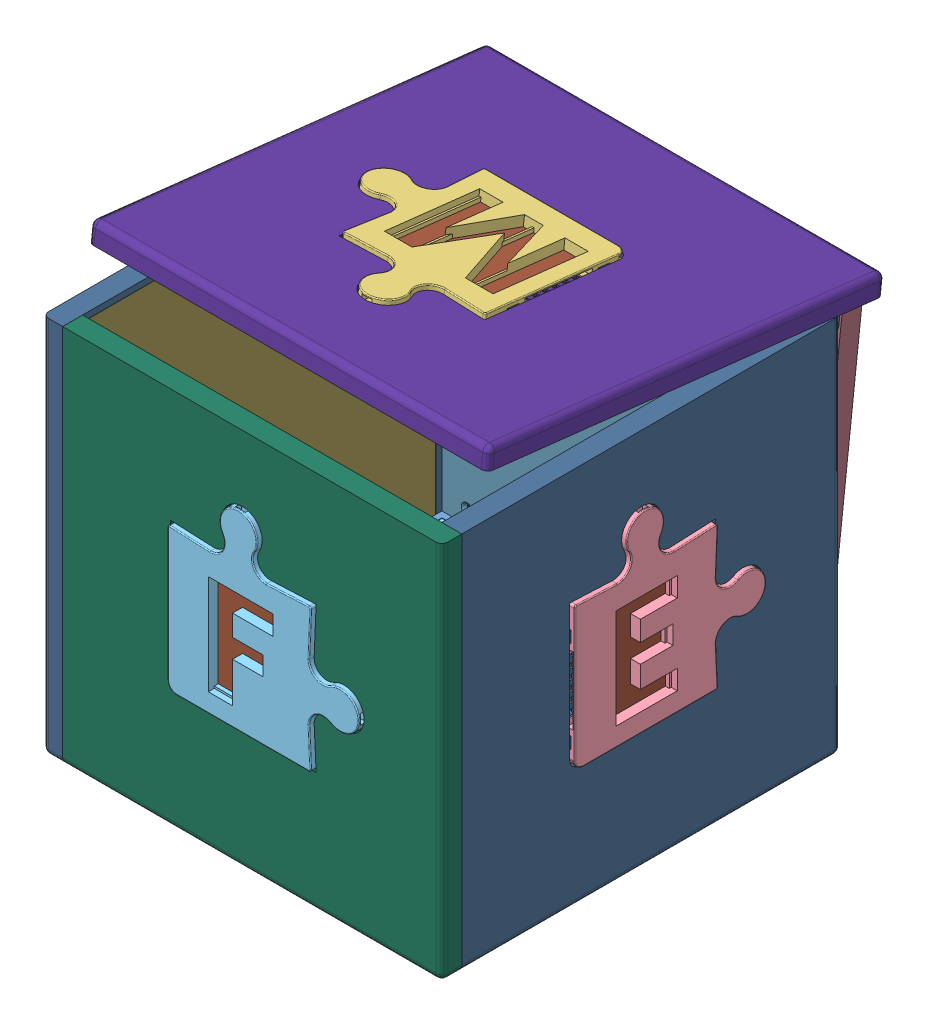
SolidWorks assembly new_full_ass, configuration Default. Lengths in mm.
Overall size (204.06 222.93 226.17).
48 component instances, 23 part files, 47 mates.
Components (placement in the parent):
- base_ass-1: base_ass [Default] at (110.6149 77.5373 125.031) size (180 19.96 180)
  - base-1: base [Default] at (-36.6134 -12.1869 24.2031) size (180 15 180)
  - speaker-2: speaker [Default] at (18.5866 0.8131 47.2031) x (0 0 -1) z (-1 0 0) size (40 8 20)
  - type-c_BMS_module-2: type-c_BMS_module [Default] at (27.2366 -9.1869 112.2031) x (0 0 -1) z (0 1 0) size (29.08 17.3 4.86)
  - battery-2: battery [Default] at (-36.6134 -10.1869 -24.7969) size (132 12 42)
  - tutup_base-1: tutup_base [Default] at (-36.6134 0.8131 24.2031) size (173.5 12 173.5)
  - switch-1: switch [Default] at (-5.9134 -5.1869 89.9531) size (10 14.96 15)
  - smart_puzzle-1: smart_puzzle [Default] at (19.033 -5.5869 172.5712) x (0 0 -1) z (0 1 0) size (76.84 76.96 8.3)
- hinge-1: hinge [Default] at (104.8865 81.1552 217.17) x (0 -1 0) z (-1 0 0) size (11.5 5 40) (flexible)
  - hinge_A-1: hinge_A [Default] at (15.8048 19.5641 50.885) size (11.5 5 40)
  - hinge_B-1: hinge_B [Default] at (6.8048 24.5641 50.885) x (-1 0 0) z (0 0 1) size (11.5 5 40)
- hinge-2: hinge [Default] at (6.0656 81.1552 180.1191) x (0 -1 0) z (0 0 -1) size (11.5 5 40) (flexible)
  - hinge_A-1: hinge_A [Default] at (15.8048 19.5641 50.885) size (11.5 5 40)
  - hinge_B-1: hinge_B [Default] at (6.8048 24.5641 50.885) x (-1 0 0) z (0 0 1) size (11.5 5 40)
- hinge-3: hinge [Default] at (43.1164 81.1552 81.2982) x (0 -1 0) z (1 0 0) size (11.99 6.27 40) (flexible)
  - hinge_A-1: hinge_A [Default] at (15.8048 19.5641 50.885) size (11.5 5 40)
  - hinge_B-1: hinge_B [Default] at (7.1444 25.5637 50.885) x (-0.993614 0.112837 0) z (0 0 1) size (11.5 5 40)
- hinge-4: hinge [Default] at (141.9374 81.1552 118.3491) x (0 -1 0) z (0 0 1) size (11.5 5 40) (flexible)
  - hinge_A-1: hinge_A [Default] at (15.8048 19.5641 50.885) size (11.5 5 40)
  - hinge_B-1: hinge_B [Default] at (6.8048 24.5641 50.885) x (-1 0 0) z (0 0 1) size (11.5 5 40)
- side_ass-2: side_ass [Default] at (-27.75 544.2015 -410.629) x (0 0 -1) z (0 -1 0) size (190 10 190)
  - side-1: side [Default] at (-559.8631 11.7515 383.8511) x (0 -1 0) z (-1 0 0) size (10 190 190)
  - RGB_backlight-1: RGB_backlight [Default] at (-559.8631 6.7515 383.8511) x (-1 0 0) z (0 0 -1) size (71 3 80)
  - tutup_side-1: tutup_side [Default] at (-564.8631 9.7515 389.9511) x (-1 0 0) z (0 0 -1) size (185.8 2 183.8)
- side_ass-3: side_ass [Default] at (175.7529 544.2015 709.0972) x (0 0 1) z (0 -1 0) size (190 10 190)
  - side-1: side [Default] at (-559.8631 11.7515 383.8511) x (0 -1 0) z (-1 0 0) size (10 190 190)
  - RGB_backlight-1: RGB_backlight [Default] at (-559.8631 6.7515 383.8511) x (-1 0 0) z (0 0 -1) size (71 3 80)
  - tutup_side-1: tutup_side [Default] at (-564.8631 9.7515 389.9511) x (-1 0 0) z (0 0 -1) size (185.8 2 183.8)
- side_top_hinge_ass-1: side_top_hinge_ass [Default] at (71.9264 168.2711 22.0939) x (0 -0.112837 -0.993614) z (-1 0 0) size (10 190 190)
  - side_top_hinge-1: side_top_hinge [Default] at (-25.2898 11.4541 -2.0751) size (10 190 190)
  - tutup_side_top_hinge-1: tutup_side_top_hinge [Default] at (-23.2898 11.4541 2.9249) x (0 0 1) z (0 -1 0) size (185.5 2 183.5)
  - RGB_backlight-1: RGB_backlight [Default] at (-23.2898 11.4541 -2.0751) x (0 0 -1) z (0 -1 0) size (71 3 80)
- side_top_magnet_ass-1: side_top_magnet_ass [Default] at (71.9462 160.3504 257.6043) x (0 0 1) z (1 0 0) size (10 190 190)
  - side_top_magnet-1: side_top_magnet [Default] at (-18.3702 0 2.0553) size (10 190 190)
  - RGB_backlight-1: RGB_backlight [Default] at (-13.3702 0 2.0553) x (0 0 1) z (0 -1 0) size (71 3 80)
  - tutup_side_top_magnet-1: tutup_side_top_magnet [Default] at (-16.3702 0 7.0553) x (0 0 1) z (0 -1 0) size (185.5 2 185.5)
- hinge-5: hinge [Default] at (43.1164 232.8688 46.0525) x (0 -0.112837 -0.993614) z (1 0 0) size (11.5 5 40) (flexible)
  - hinge_A-1: hinge_A [Default] at (15.8048 19.5641 50.885) size (11.5 5 40)
  - hinge_B-1: hinge_B [Default] at (6.8048 24.5641 50.885) x (-1 0 0) z (0 0 1) size (11.5 5 40)
- top_ass-1: top_ass [Default] at (54.7211 254.2163 143.7349) x (0 0.993614 -0.112837) z (-1 0 0) size (10 200 200)
  - top-1: top [Default] at (11.8751 15.2721 -19.2804) size (10 200 200)
  - tutup_top-1: tutup_top [Default] at (13.8751 15.2721 -19.2804) x (0 0 1) z (0 -1 0) size (195.5 2 193.5)
  - RGB_backlight-1: RGB_backlight [Default] at (16.8751 15.2721 -19.2804) x (0 0 1) z (0 -1 0) size (71 3 80)
- A-1: A [Default] at (-22.9985 161.3504 149.2341) x (0 0 1) z (0 -1 0) size (95.8 5.06 95.8)
- H-1: H [Default] at (74.0015 159.9475 41.4465) x (-1 0 0) z (0 -0.993614 0.112837) size (95.8 5.06 95.8)
- M-1: M [Default] at (74.0015 271.3604 127.4241) x (-1 0 0) z (0 -0.112837 -0.993614) size (95.8 5.06 95.8)
- E-1: E [Default] at (171.0015 161.3504 149.2341) x (0 0 -1) z (0 -1 0) size (95.8 5.06 95.8)
- N-1: N [Default] at (74.0015 161.3504 246.2341) x (1 0 0) z (0 -1 0) size (95.8 5.06 95.8)
Mates (geometry in assembly coordinates):
- Coincident1: coincident anti-aligned: line of base_ass-1/base-1 through (94.4015 65.3504 239.2341) axis (1 0 0); line of hinge-1 through (91.3609 65.3504 239.2341) axis (-1 0 0)
- Parallel1: parallel anti-aligned: plane of base_ass-1/base-1 through (74.0015 65.3504 236.6341) normal (0 0 1); plane of hinge-1/hinge_A-1 through (54.0015 65.3504 236.7341) normal (0 0 -1)
- Width1: width anti-aligned: plane of base_ass-1/base-1 through (53.6015 65.3504 236.6341) normal (1 0 0); plane of hinge-1/hinge_A-1 through (94.4015 65.3504 236.6341) normal (-1 0 0); plane of base_ass-1/base-1 through (54.0015 74.3504 239.2341) normal (-1 0 0); plane of hinge-1/hinge_A-1 through (94.0015 74.3504 239.2341) normal (1 0 0)
- Coincident3: coincident anti-aligned: line of base_ass-1/base-1 through (-15.9985 65.3504 59.2341) axis (0 0 1); line of hinge-2 through (-15.9985 65.3504 166.5936) axis (0 0 -1)
- Parallel2: parallel anti-aligned: plane of base_ass-1/base-1 through (-13.3985 65.3504 149.2341) normal (-1 0 0); plane of hinge-2/hinge_A-1 through (-13.4985 65.3504 129.2341) normal (1 0 0)
- Width2: width anti-aligned: plane of base_ass-1/base-1 through (-13.3985 65.3504 128.8341) normal (0 0 1); plane of hinge-2/hinge_A-1 through (-13.3985 65.3504 169.6341) normal (0 0 -1); plane of base_ass-1/base-1 through (-15.9985 74.3504 129.2341) normal (0 0 -1); plane of hinge-2/hinge_A-1 through (-15.9985 74.3504 169.2341) normal (0 0 1)
- Coincident5: coincident aligned: line of base_ass-1/base-1 through (94.4015 65.3504 59.2341) axis (1 0 0); line of hinge-3 through (56.642 65.3504 59.2341) axis (1 0 0)
- Parallel3: parallel anti-aligned: plane of base_ass-1/base-1 through (74.0015 65.3504 61.8341) normal (0 0 -1); plane of hinge-3/hinge_A-1 through (94.0015 65.3504 61.7341) normal (0 0 1)
- Width3: width anti-aligned: plane of base_ass-1/base-1 through (94.4015 65.3504 61.8341) normal (-1 0 0); plane of hinge-3/hinge_A-1 through (53.6015 65.3504 61.8341) normal (1 0 0); plane of base_ass-1/base-1 through (94.0015 74.3504 59.2341) normal (1 0 0); plane of hinge-3/hinge_A-1 through (54.0015 74.3504 59.2341) normal (-1 0 0)
- Coincident11: coincident aligned: line of base_ass-1/base-1 through (164.0015 65.3504 169.6341) axis (0 0 1); line of hinge-4 through (164.0015 65.3504 131.8746) axis (0 0 1)
- Width4: width anti-aligned: plane of base_ass-1/base-1 through (161.4015 65.3504 128.8341) normal (0 0 1); plane of hinge-4/hinge_A-1 through (161.4015 65.3504 169.6341) normal (0 0 -1); plane of base_ass-1/base-1 through (164.0015 74.3504 129.2341) normal (0 0 -1); plane of hinge-4/hinge_A-1 through (164.0015 74.3504 169.2341) normal (0 0 1)
- Parallel5: parallel anti-aligned: plane of base_ass-1/base-1 through (161.4015 65.3504 149.2341) normal (1 0 0); plane of hinge-4/hinge_A-1 through (161.5015 65.3504 169.2341) normal (-1 0 0)
- Width5: width anti-aligned: plane of side_ass-2/side-1 through (-18.5985 65.3504 128.8341) normal (0 0 1); plane of hinge-2/hinge_B-1 through (-18.5985 65.3504 169.6341) normal (0 0 -1); plane of side_ass-2/side-1 through (-15.9985 74.3504 129.2341) normal (0 0 -1); plane of hinge-2/hinge_B-1 through (-15.9985 74.3504 169.2341) normal (0 0 1)
- Parallel6: parallel anti-aligned: plane of hinge-2/hinge_B-1 through (-18.4985 74.3504 129.2341) normal (-1 0 0); plane of side_ass-2/side-1 through (-18.5985 160.3504 149.2341) normal (1 0 0)
- Coincident12: coincident aligned: line of base_ass-1/base-1 through (-15.9985 65.3504 169.6341) axis (0 0 1); line of side_ass-2/side-1 through (-15.9985 65.3504 169.6341) axis (0 0 1)
- Width6: width anti-aligned: plane of side_ass-3/side-1 through (166.6015 65.3504 128.8341) normal (0 0 1); plane of hinge-4/hinge_B-1 through (166.6015 65.3504 169.6341) normal (0 0 -1); plane of side_ass-3/side-1 through (164.0015 74.3504 129.2341) normal (0 0 -1); plane of hinge-4/hinge_B-1 through (164.0015 74.3504 169.2341) normal (0 0 1)
- Parallel7: parallel anti-aligned: plane of hinge-4/hinge_B-1 through (166.5015 74.3504 169.2341) normal (1 0 0); plane of side_ass-3/side-1 through (166.6015 160.3504 149.2341) normal (-1 0 0)
- Coincident14: coincident anti-aligned: line of base_ass-1/base-1 through (164.0015 65.3504 169.6341) axis (0 0 1); line of side_ass-3/side-1 through (164.0015 65.3504 239.2341) axis (0 0 -1)
- Width7: width anti-aligned: plane of side_top_hinge_ass-1/side_top_hinge-1 through (94.4015 65.0571 56.6507) normal (-1 0 0); plane of hinge-3/hinge_B-1 through (53.6015 65.0571 56.6507) normal (1 0 0); plane of side_top_hinge_ass-1/side_top_hinge-1 through (94.0015 74.293 58.2186) normal (1 0 0); plane of hinge-3/hinge_B-1 through (54.0015 74.293 58.2186) normal (-1 0 0)
- Parallel8: parallel anti-aligned: plane of hinge-3/hinge_B-1 through (94.0015 74.0109 55.7345) normal (0 -0.112837 -0.993614); plane of side_top_hinge_ass-1/side_top_hinge-1 through (74.0015 159.4503 45.9312) normal (0 0.112837 0.993614)
- Coincident16: coincident anti-aligned: line of base_ass-1/base-1 through (-15.9985 65.3504 59.2341) axis (1 0 0); line of side_top_hinge_ass-1/side_top_hinge-1 through (53.6015 65.3504 59.2341) axis (-1 0 0)
- Width8: width anti-aligned: plane of side_top_magnet_ass-1/side_top_magnet-1 through (94.4015 65.3504 241.8341) normal (-1 0 0); plane of hinge-1/hinge_B-1 through (53.6015 65.3504 241.8341) normal (1 0 0); plane of side_top_magnet_ass-1/side_top_magnet-1 through (94.0015 74.3504 239.2341) normal (1 0 0); plane of hinge-1/hinge_B-1 through (54.0015 74.3504 239.2341) normal (-1 0 0)
- Parallel9: parallel anti-aligned: plane of hinge-1/hinge_B-1 through (54.0015 74.3504 241.7341) normal (0 0 1); plane of side_top_magnet_ass-1/side_top_magnet-1 through (74.0015 160.3504 241.8341) normal (0 0 -1)
- Coincident17: coincident aligned: line of base_ass-1/base-1 through (-15.9985 65.3504 239.2341) axis (1 0 0); line of side_top_magnet_ass-1/side_top_magnet-1 through (-15.9985 65.3504 239.2341) axis (1 0 0)
- Width9: width anti-aligned: plane of side_top_hinge_ass-1/side_top_hinge-1 through (94.4015 251.4633 37.2936) normal (-1 0 0); plane of hinge-5/hinge_A-1 through (53.6015 251.4633 37.2936) normal (1 0 0); plane of side_top_hinge_ass-1/side_top_hinge-1 through (94.0015 254.0242 36.8015) normal (1 0 0); plane of hinge-5/hinge_A-1 through (54.0015 254.0242 36.8015) normal (-1 0 0)
- Parallel10: parallel anti-aligned: plane of side_top_hinge_ass-1/side_top_hinge-1 through (74.0015 251.5536 38.0885) normal (0 0.993614 -0.112837); plane of hinge-5/hinge_A-1 through (94.0015 250.5246 28.1411) normal (0 -0.993614 0.112837)
- Coincident19: coincident aligned: line of side_top_hinge_ass-1/side_top_hinge-1 through (94.4015 253.0086 27.859) axis (1 0 0); line of hinge-5 through (56.642 253.0086 27.859) axis (1 0 0)
- Width10: width aligned: plane of top_ass-1/top-1 through (53.6015 255.592 27.5656) normal (1 0 0); plane of hinge-5/hinge_B-1 through (94.4015 255.592 27.5656) normal (-1 0 0); plane of top_ass-1/top-1 through (94.0015 254.0242 36.8015) normal (1 0 0); plane of hinge-5/hinge_B-1 through (54.0015 254.0242 36.8015) normal (-1 0 0)
- Parallel11: parallel anti-aligned: plane of hinge-5/hinge_B-1 through (94.0015 256.5082 36.5194) normal (0 0.993614 -0.112837); plane of top_ass-1/top-1 through (74.0015 266.8757 126.927) normal (0 -0.993614 0.112837)
- Coincident21: coincident anti-aligned: line of side_top_hinge_ass-1/side_top_hinge-1 through (-22.9985 253.0086 27.859) axis (1 0 0); line of top_ass-1/top-1 through (53.6015 253.0086 27.859) axis (-1 0 0)
- Width11: width anti-aligned: plane of side_ass-2/side-1 through (-22.9985 197.3504 135.092) normal (0 -0.998955 -0.045702); plane of side_ass-2/side-1 through (-22.9985 125.3504 118.2341) normal (0 1 0); plane of A-1 through (-27.9985 196.7504 135.0779) normal (0 0.998955 0.045702); plane of A-1 through (-27.9985 125.9504 118.2341) normal (0 -1 0)
- Width12: width aligned: plane of side_ass-2/side-1 through (-22.9985 130.3504 113.2341) normal (0 0 1); plane of side_ass-2/side-1 through (-22.9985 146.2083 185.2341) normal (0 -0.047889 -0.998853); plane of A-1 through (-27.9985 125.9504 185.6046) normal (0 0.047889 0.998853); plane of A-1 through (-27.9985 197.7224 113.8341) normal (0 0 -1)
- Coincident22: coincident anti-aligned: line of side_ass-2/side-1 through (-25.9985 255.3504 59.2341) axis (0 -1 0); line of side_top_hinge_ass-1/side_top_hinge-1 through (-25.9985 68.3504 59.2341) axis (0 1 0)
- Coincident23: coincident anti-aligned: plane of side_ass-2/side-1 through (-22.9985 130.3504 118.2341) normal (-1 0 0); plane of A-1 through (-22.9985 130.3504 118.2341) normal (1 0 0)
- Width13: width anti-aligned: plane of side_top_hinge_ass-1/side_top_hinge-1 through (110.0015 129.1455 44.9444) normal (-1 0 0); plane of side_top_hinge_ass-1/side_top_hinge-1 through (37.0015 196.7112 37.2715) normal (0.999123 0.041611 -0.004725); plane of H-1 through (109.4015 195.5229 32.3743) normal (1 0 0); plane of H-1 through (38.6015 172.4543 34.994) normal (-0.999123 -0.041611 0.004725)
- Width14: width aligned: plane of side_top_hinge_ass-1/side_top_hinge-1 through (59.8593 195.7176 37.3844) normal (-0.043707 -0.992664 0.112729); plane of side_top_hinge_ass-1/side_top_hinge-1 through (105.0015 124.1774 45.5086) normal (0 0.993614 -0.112837); plane of H-1 through (105.0015 124.2094 40.4728) normal (0 -0.993614 0.112837); plane of H-1 through (37.6283 195.523 32.3743) normal (0.043707 0.992664 -0.112729)
- Coincident24: coincident anti-aligned: plane of side_top_hinge_ass-1/side_top_hinge-1 through (105.0015 129.1455 44.9444) normal (0 -0.112837 -0.993614); plane of H-1 through (105.0015 129.1455 44.9444) normal (0 0.112837 0.993614)
- Width15: width anti-aligned: plane of top_ass-1/top-1 through (59.8593 275.4226 163.1942) normal (-0.043707 -0.112729 -0.992664); plane of top_ass-1/top-1 through (105.0015 267.2983 91.654) normal (0 0.112837 0.993614); plane of M-1 through (37.6283 280.4326 162.9996) normal (0.043707 0.112729 0.992664); plane of M-1 through (105.0015 272.3341 91.686) normal (0 -0.112837 -0.993614)
- Width16: width anti-aligned: plane of top_ass-1/top-1 through (110.0015 267.8625 96.6221) normal (-1 0 0); plane of top_ass-1/top-1 through (38.0015 269.6519 112.3787) normal (0.998853 -0.005404 -0.047583); plane of M-1 through (109.4015 280.4326 162.9995) normal (1 0 0); plane of M-1 through (37.6309 272.3341 91.686) normal (-0.998853 0.005404 0.047583)
- Parallel12: parallel anti-aligned: line of side_ass-2/side-1 through (-25.9985 255.3504 246.2341) axis (0 0 -1); line of top_ass-1/top-1 through (-25.9985 255.3504 52.2341) axis (0 0 1)
- Coincident26: coincident anti-aligned: plane of top_ass-1/top-1 through (105.0015 267.8625 96.6221) normal (0 0.993614 -0.112837); plane of M-1 through (105.0015 267.8625 96.6221) normal (0 -0.993614 0.112837)
- Width17: width anti-aligned: plane of side_ass-3/side-1 through (171.0015 197.3504 163.3762) normal (0 -0.998955 0.045702); plane of side_ass-3/side-1 through (171.0015 125.3504 180.2341) normal (0 1 0); plane of E-1 through (176.0015 196.7504 163.3903) normal (0 0.998955 -0.045702); plane of E-1 through (176.0015 125.9504 180.2341) normal (0 -1 0)
- Width18: width anti-aligned: plane of side_ass-3/side-1 through (171.0015 130.3504 185.2341) normal (0 0 -1); plane of side_ass-3/side-1 through (171.0015 198.3504 112.2341) normal (0 0.041878 0.999123); plane of E-1 through (176.0015 197.7224 184.6341) normal (0 0 1); plane of E-1 through (176.0015 174.5054 113.8341) normal (0 -0.041878 -0.999123)
- Coincident27: coincident anti-aligned: plane of side_ass-3/side-1 through (171.0015 130.3504 180.2341) normal (1 0 0); plane of E-1 through (171.0015 130.3504 180.2341) normal (-1 0 0)
- Width19: width anti-aligned: plane of side_top_magnet_ass-1/side_top_magnet-1 through (59.8593 197.3504 246.2341) normal (-0.045702 -0.998955 0); plane of side_top_magnet_ass-1/side_top_magnet-1 through (43.0015 125.3504 246.2341) normal (0 1 0); plane of N-1 through (59.8453 196.7504 251.2341) normal (0.045702 0.998955 0); plane of N-1 through (43.0015 125.9504 251.2341) normal (0 -1 0)
- Width20: width anti-aligned: plane of side_top_magnet_ass-1/side_top_magnet-1 through (38.0015 130.3504 246.2341) normal (1 0 0); plane of side_top_magnet_ass-1/side_top_magnet-1 through (110.0015 146.2083 246.2341) normal (-0.998853 -0.047889 0); plane of N-1 through (38.6015 197.7224 251.2341) normal (-1 0 0); plane of N-1 through (110.372 125.9504 251.2341) normal (0.998853 0.047889 0)
- Coincident28: coincident anti-aligned: plane of side_top_magnet_ass-1/side_top_magnet-1 through (43.0015 130.3504 246.2341) normal (0 0 1); plane of N-1 through (43.0015 130.3504 246.2341) normal (0 0 -1)
